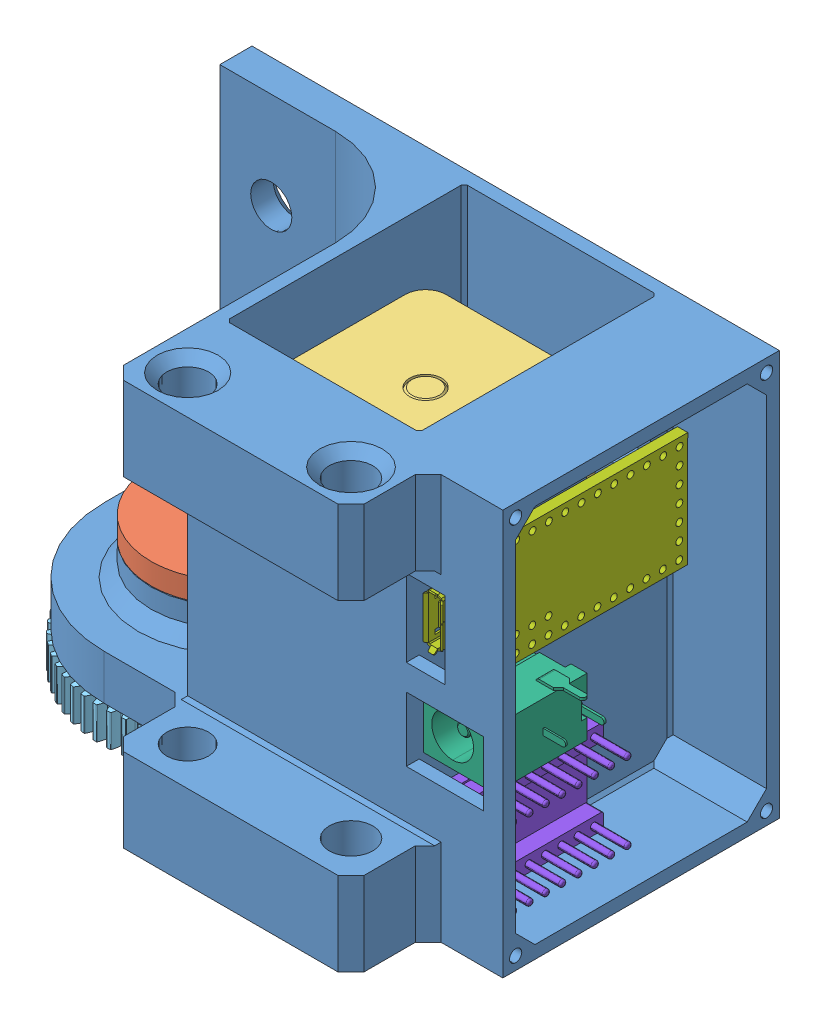
SolidWorks assembly commutator, configuration Default. Lengths in mm.
Overall size (90.87 70.48 60.87).
8 component instances, 8 part files, 4 mates.
Components (placement in the parent):
- rf_commutator_housing-1: rf_commutator_housing [Default] at origin size (82 63 55)
- Fairview_FMRJ1002_rf_rotary_jpint_female_to_female_flanged-1: Fairview_FMRJ1002_rf_rotary_jpint_female_to_female_flanged [Default] at (0 10.1486 0) x (0 -1 0) z (-0.521112 0 0.853488) size (34.7 25.4 25.4)
- 6627T370_POSITION-CONTROL DC MOTOR-1: 6627T370_POSITION-CONTROL DC MOTOR [6627T37] at (30 13.5246 0) x (0 0 -1) z (0 -1 0) size (28.19 28.19 52.07)
- gear_a-2: gear_a [Default] at (30 -2.3438 0) x (0.979702 0 -0.200458) z (0 -1 0) size (21.12 21.05 5.08)
- gear_b-2: gear_b [Default] at (0 -2.3568 0) x (0.670791 0 0.741646) z (0 -1 0) size (40.88 40.88 13.12)
- CUI_PJ-102A-2: CUI_PJ-102A [Default] at (58.3028 18.2997 9.8994) x (0 -1 0) z (0 0 -1) size (9.4 14.5 14.4)
- Teensy_lc-2: Teensy_lc [Default] at (52.8125 23.9482 17.6843) x (0 1 0) z (-1 0 0) size (17.93 36.98 4.49)
- DRV 8825 With Headers Assem-1: DRV 8825 With Headers Assem [Default] at (67.8565 -6.9624 -1.3078) x (0 0 1) z (-1 0 0) size (21 15 10.9)
Mates (geometry in assembly coordinates):
- Concentric1: concentric: cylinder of rf_commutator_housing-1 through (0 5 0) axis (0 -1 0) radius 7.5; cylinder of Fairview_FMRJ1002_rf_rotary_jpint_female_to_female_flanged-1 through (0 13.4486 0) axis (0 1 0) radius 3.1336
- Concentric2: concentric: cylinder of rf_commutator_housing-1 through (30 5 0) axis (0 -1 0) radius 12.5; cylinder of 6627T370_POSITION-CONTROL DC MOTOR-1 through (30 13.5246 0) axis (0 1 0) radius 10.9982
- Concentric8: concentric: cylinder of Fairview_FMRJ1002_rf_rotary_jpint_female_to_female_flanged-1 through (0 13.4486 0) axis (0 1 0) radius 12.7; cylinder of gear_b-2 through (0 -2.3568 0) axis (0 -1 0) radius 6.095
- Concentric9: concentric: cylinder of 6627T370_POSITION-CONTROL DC MOTOR-1 through (30 -6.5414 0) axis (0 -1 0) radius 2.4994; cylinder of gear_a-2 through (30 -2.3438 0) axis (0 -1 0) radius 2.5
